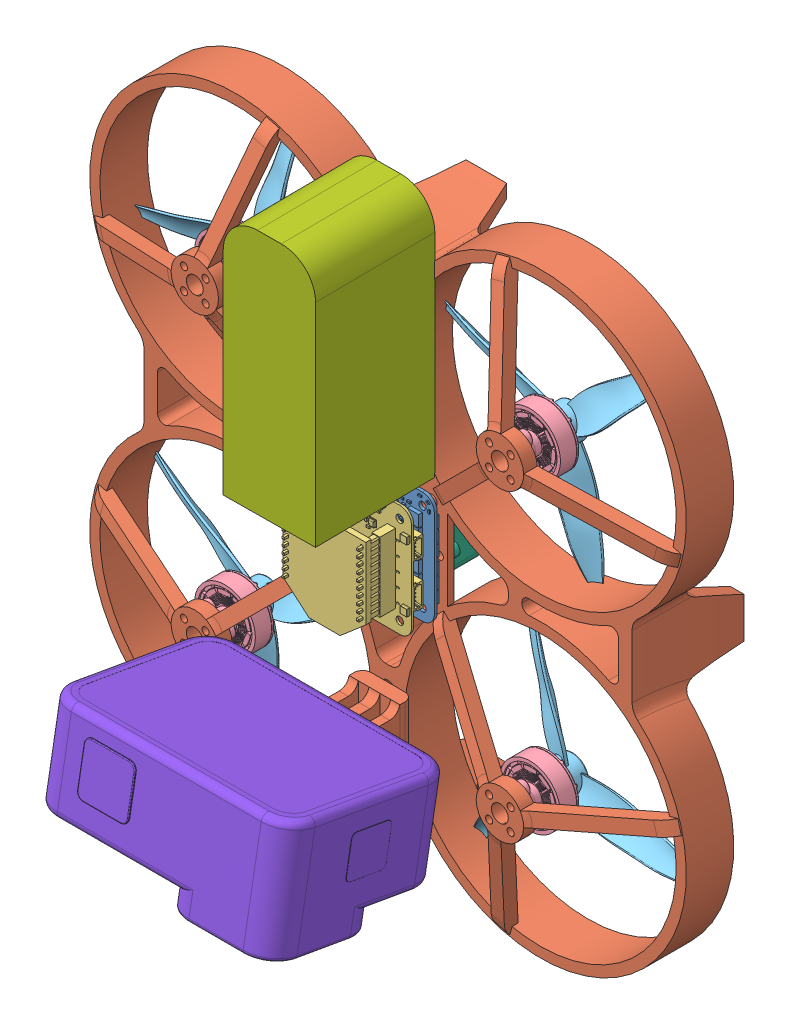
SolidWorks assembly Quad_assem, configuration Default. Lengths in mm.
Overall size (176 179.73 101.1).
14 component instances, 8 part files, 26 mates.
Components (placement in the parent):
- 4in1_ESC-1: 4in1_ESC [Default] at (-19 -71.0915 82.7585) x (-1 0 0) z (0 0 1) size (33 33 7.6)
- Quad-1: Quad [Default] at (-19 -71.0915 50.9225) x (-1 0 0) z (0 1 0) size (176 48 176)
- FlightController.step-1: FlightController.step [Default] at (-19 -71.0915 89.4622) x (-1 0 0) z (0 0 1) size (33 33 15.78)
- 1404 motor.step-5: 1404 motor.step [Default] at (26 -116.0915 87.9225) x (-0.963387 0.268113 0) z (0 0 -1) size (17.9 17.9 14.53)
- Prop-1: Prop [Default] at (26 -116.0915 73.1725) x (-0.291728 0.956501 0) z (-0.956501 -0.291728 0) size (58.53 5.95 67.58)
- Prop-2: Prop [Default] at (-64 -116.0915 73.1725) x (-0.052615 -0.998615 0) z (0.998615 -0.052615 0) size (58.53 5.95 67.58)
- 1404 motor.step-6: 1404 motor.step [Default] at (-64 -116.0915 87.9225) x (0.296226 -0.955118 0) z (0 0 -1) size (17.9 17.9 14.53)
- Prop-3: Prop [Default] at (26 -26.0915 73.1725) x (-0.951505 0.307634 0) z (-0.307634 -0.951505 0) size (58.53 5.95 67.58)
- 1404 motor.step-7: 1404 motor.step [Default] at (26 -26.0915 87.9225) x (0.40894 0.912561 0) z (0 0 -1) size (17.9 17.9 14.53)
- Prop-4: Prop [Default] at (-64 -26.0915 73.1725) x (-0.967559 -0.252646 0) z (0.252646 -0.967559 0) size (58.53 5.95 67.58)
- 1404 motor.step-8: 1404 motor.step [Default] at (-64 -26.0915 87.9225) x (0.79493 0.606701 0) z (0 0 -1) size (17.9 17.9 14.53)
- ToF-1: ToF [Default] at (-19 -71.0915 77.9225) x (1 0 0) z (0 1 0) size (34.5 13.5 18.5)
- Battery-1: Battery [Default] at (-5.1578 -15.66 97.5484) x (0 -1 0) z (-0.999962 0 0.008727) size (72.6 35.5 27)
- GoPro Hero 9-1: GoPro Hero 9 [Default] at (-54.2908 -97.3374 145.6937) x (1 0 0) z (0 -0.173648 -0.984808) size (72.1 33.6 50.5)
Mates (geometry in assembly coordinates):
- Concentric3: concentric aligned: circle of 4in1_ESC-1; circle of FlightController.step-1
- Concentric4: concentric aligned: circle of 4in1_ESC-1; circle of FlightController.step-1
- Distance3: distance = 6.08 mm anti-aligned: plane of 4in1_ESC-1 through (-2.5 -58.0915 82.7585) normal (0 0 1); plane of FlightController.step-1 through (-2.5 -58.0915 88.8385) normal (0 0 -1)
- Concentric5: concentric aligned: circle of 1404 motor.step-5; circle of Prop-1
- Concentric6: concentric aligned: circle of Prop-2; circle of 1404 motor.step-6
- Concentric7: concentric aligned: circle of Prop-3; circle of 1404 motor.step-7
- Concentric8: concentric aligned: circle of Prop-4; circle of 1404 motor.step-8
- Coincident11: coincident aligned: plane of Quad-1 through (0 -71.0915 79.9225) normal (1 0 0)
- Coincident17: coincident anti-aligned: plane of Prop-4 through (-64 -26.0915 75.9225) normal (0 0 1); plane of 1404 motor.step-8 through (-64 -26.0915 75.9225) normal (0 0 -1)
- Coincident18: coincident anti-aligned: plane of Prop-3 through (26 -26.0915 75.9225) normal (0 0 1); plane of 1404 motor.step-7 through (26 -26.0915 75.9225) normal (0 0 -1)
- Coincident19: coincident anti-aligned: plane of Prop-2 through (-64 -116.0915 75.9225) normal (0 0 1); plane of 1404 motor.step-6 through (-64 -116.0915 75.9225) normal (0 0 -1)
- Coincident20: coincident anti-aligned: plane of 1404 motor.step-5 through (26 -116.0915 75.9225) normal (0 0 -1); plane of Prop-1 through (26 -116.0915 75.9225) normal (0 0 1)
- Coincident21: coincident anti-aligned: plane of Quad-1 through (26 -116.0915 87.9225) normal (0 0 -1); plane of 1404 motor.step-5 through (26 -116.0915 87.9225) normal (0 0 1)
- Coincident22: coincident anti-aligned: plane of Quad-1 through (26 -26.0915 87.9225) normal (0 0 -1); plane of 1404 motor.step-7 through (26 -26.0915 87.9225) normal (0 0 1)
- Coincident23: coincident anti-aligned: plane of Quad-1 through (-64 -26.0915 87.9225) normal (0 0 -1); plane of 1404 motor.step-8 through (-64 -26.0915 87.9225) normal (0 0 1)
- Coincident24: coincident anti-aligned: plane of Quad-1 through (-64 -116.0915 87.9225) normal (0 0 -1); plane of 1404 motor.step-6 through (-64 -116.0915 87.9225) normal (0 0 1)
- Concentric9: concentric aligned: circle of Quad-1; circle of 1404 motor.step-7
- Concentric10: concentric aligned: circle of Quad-1; circle of 1404 motor.step-5
- Concentric11: concentric aligned: circle of Quad-1; circle of 1404 motor.step-6
- Concentric12: concentric aligned: circle of Quad-1; circle of 1404 motor.step-8
- Coincident27: coincident anti-aligned: plane of Quad-1 through (-4.5 -56.5915 77.9225) normal (0 0 -1); plane of ToF-1 through (-8.3 -64.3415 77.9225) normal (0 0 1)
- Concentric15: concentric anti-aligned: circle of Quad-1; circle of ToF-1
- Concentric16: concentric anti-aligned: circle of Quad-1; circle of ToF-1
- Concentric17: concentric aligned: circle of 4in1_ESC-1; circle of Quad-1
- Concentric18: concentric aligned: circle of Quad-1; circle of FlightController.step-1
- Coincident33: coincident anti-aligned: plane of 4in1_ESC-1 through (-2.5 -58.0915 81.9225) normal (0 0 -1); plane of Quad-1 through (-6 -84.0915 81.9225) normal (0 0 1)
